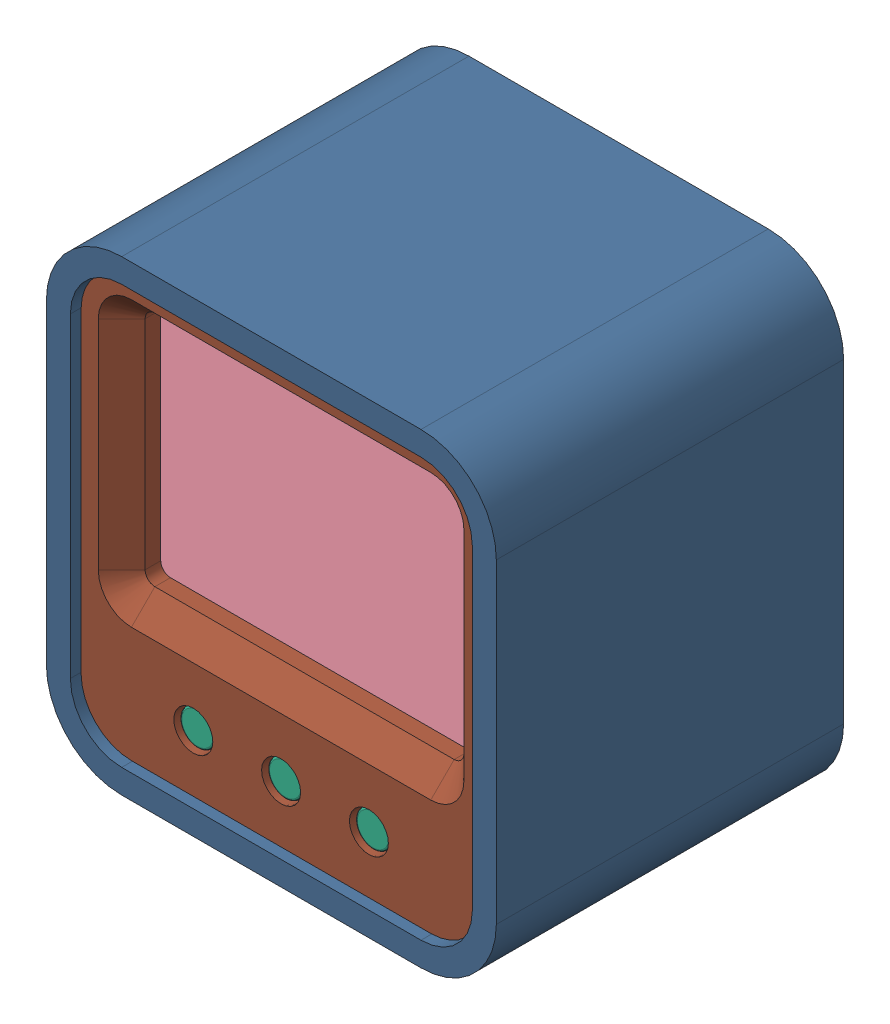
SolidWorks assembly 方案4, configuration 默认. Lengths in mm.
Overall size (23.06 23.9 17.8).
20 component instances, 11 part files, 6 mates.
Components (placement in the parent):
- SAU-G0+EX_AHT-GL_PCB-1: SAU-G0+EX_AHT-GL_PCB [默认] at (-21.4442 -48.8573 14.6489) size (20.36 19.5 16.16)
  - SAU-G0_PCB-1: SAU-G0_PCB [默认] at (11.5169 60.6772 -14.7107) size (20.36 19.5 15.06)
    - SAU-G0_STEP_AD-1: SAU-G0_STEP_AD [默认] at (-16.5787 -13.328 24.4103) size (18.66 19.5 12.19)
    - 2.00mm_2x2_垫板PCB_厚1.0mm-1: 2.00mm_2x2_垫板PCB_厚1.0mm [默认] at (3.1013 6.262 22.4106) x (1 0 0) z (0 -1 0) size (4.5 1 4.5)
    - 2.00mm母座2x2-1: 2.00mm母座2x2 [Default] at (4.1013 6.262 18.1106) x (1 0 0) z (0 1 0) size (4.5 7.1 4.5)
    - 2.00mm_2x2_垫板PCB_厚1.0mm-2: 2.00mm_2x2_垫板PCB_厚1.0mm [默认] at (-10.8587 6.262 22.4106) x (-1 0 0) z (0 1 0) size (4.5 1 4.5)
    - 2.00mm母座2x2-2: 2.00mm母座2x2 [Default] at (-11.8587 6.262 18.1106) x (-1 0 0) z (0 -1 0) size (4.5 7.1 4.5)
    - 0.66寸_64x48_TOP_FPC背面距离背板1mm-1: 0.66寸_64x48_TOP_FPC背面距离背板1mm [Default] at (-3.8787 8.514 25.9703) x (1 0 0) z (0 -1 0) size (18.46 2.27 19.3)
    - 轻触开关+柔性PCB-1: 轻触开关+柔性PCB [默认] at (-0.958 10.42 26.3367) x (1 0 0) z (0 -1 0) size (20.26 5.16 4.01)
      - 方案2-轻触开关_柔性PCB-1: 方案2-轻触开关_柔性PCB [默认] at (-12.1506 0.4339 17.21) size (20.26 3.56 4.01)
      - 轻触开关3x3.5x1.5_3x4.0x2.0-1: 轻触开关3x3.5x1.5_3x4.0x2.0 [默认] at (-2.9206 0.5339 19.31) size (4 1.6 3.4)
      - 轻触开关3x3.5x1.5_3x4.0x2.0-2: 轻触开关3x3.5x1.5_3x4.0x2.0 [默认] at (1.5794 0.5339 19.31) size (4 1.6 3.4)
      - 轻触开关3x3.5x1.5_3x4.0x2.0-3: 轻触开关3x3.5x1.5_3x4.0x2.0 [默认] at (-7.4206 0.5339 19.31) size (4 1.6 3.4)
  - SAU-G0-EX_AHT-GL_PCB-1: SAU-G0-EX_AHT-GL_PCB [默认] at (7.6382 62.4703 19.0392) x (-1 0 0) z (0 0 -1) size (18.66 19.5 9.5)
    - SAU-G0-EX_AHT-GL_STEP_AD-1: SAU-G0-EX_AHT-GL_STEP_AD [默认] at (33.02 -15.1211 17.6394) x (-1 0 0) z (0 0 -1) size (18.66 19.5 3.8)
    - 2.0mm排针2x2-1: 2.0mm排针2x2 [Default] at (-7.9796 3.4685 17.6394) x (-1 0 0) z (0 -1 0) size (4 8.2 4)
    - 2.0mm排针2x2-2: 2.0mm排针2x2 [Default] at (7.9796 5.4685 17.6394) x (1 0 0) z (0 1 0) size (4 8.2 4)
  - 601419(18.5x13.5x6.2mm)_3.7V_100mAh-1: 601419(18.5x13.5x6.2mm)_3.7V_100mAh [Default] at (16.9702 57.9392 3.2499) x (0 -1 0) z (-1 0 0) size (13.5 6.2 18)
- 外壳-方案2-1: 外壳-方案2 [默认] at (-13.806 -1.2661 28.6185) size (23.06 23.9 17.8)
- 外壳-方案2-盖子-1: 外壳-方案2-盖子 [默认] at (-13.806 -1.2661 28.6185) size (20.8 21.64 2)
Mates (geometry in assembly coordinates):
- 重合3: coincident anti-aligned: plane of SAU-G0+EX_AHT-GL_PCB-1/SAU-G0_PCB-1/0.66寸_64x48_TOP_FPC背面距离背板1mm-1 through (-13.806 20.3339 26.6185) normal (0 0 1); plane of 外壳-方案2-1 through (-13.806 -1.2661 26.6185) normal (0 0 -1)
- 距离1: distance = 0.2 mm anti-aligned: plane of 外壳-方案2-1 through (-4.276 20.6339 -10.7458) normal (0 -1 0); plane of SAU-G0+EX_AHT-GL_PCB-1/SAU-G0_PCB-1/SAU-G0_STEP_AD-1 through (-23.138 20.4339 23.3488) normal (0 1 0)
- 重合5: coincident aligned: plane of SAU-G0+EX_AHT-GL_PCB-1/SAU-G0_PCB-1 through (-13.806 11.8199 -0.0618) normal (1 0 0); plane of 外壳-方案2-1 through (-13.806 -1.2661 28.6185) normal (1 0 0)
- 重合6: coincident: line of SAU-G0+EX_AHT-GL_PCB-1/SAU-G0_PCB-1/0.66寸_64x48_TOP_FPC背面距离背板1mm-1 through (-5.076 19.8339 26.6185) axis (-1 0 0); plane of 外壳-方案2-盖子-1 through (-13.806 -1.2661 26.6185) normal (0 0 -1)
- 同心1: concentric aligned: cylinder of 外壳-方案2-盖子-1 through (-6.136 18.7739 11.3185) axis (0 0 1) radius 2.5804; cylinder of 外壳-方案2-1 through (-6.136 18.7739 11.3185) axis (0 0 1) radius 3.86
- 同心2: concentric aligned: cylinder of 外壳-方案2-1 through (-6.136 2.5939 11.3185) axis (0 0 1) radius 3.86; cylinder of 外壳-方案2-盖子-1 through (-6.136 2.5939 11.3185) axis (0 0 1) radius 2.5804
